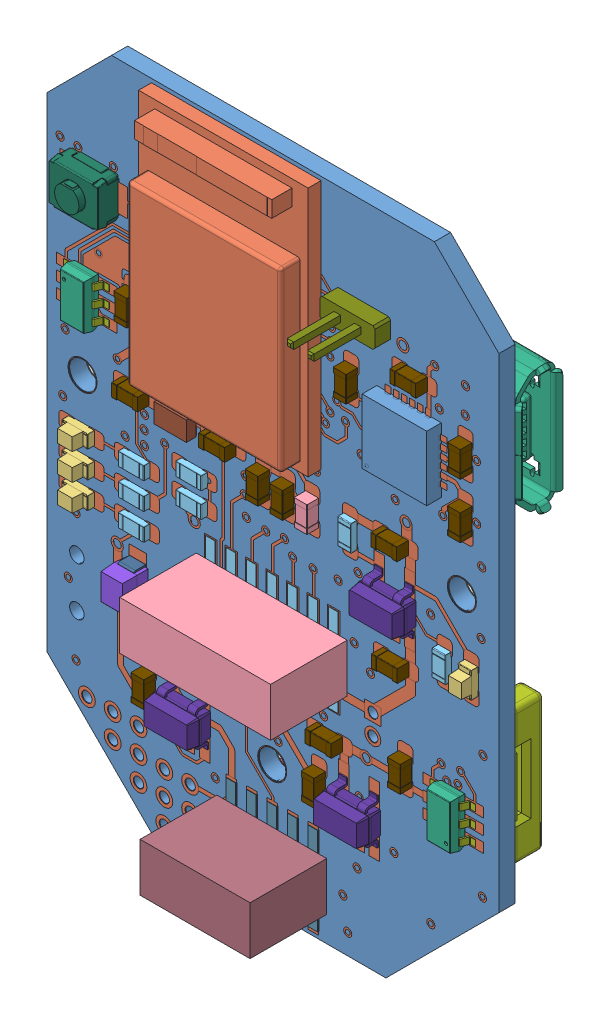
SolidWorks assembly mainboard, configuration Default. Lengths in mm.
Overall size (28.95 41 10.7).
78 component instances, 27 part files, 2 mates.
Components (placement in the parent):
- Board_Geoms_6845.step-1: Board_Geoms_6845.step [Default] at origin size (28 41 1.11)
  - Pcb_6845.step-1: Pcb_6845.step [Default] at (-183 131 0) size (28 41 1)
  - topTracks_6845.step-1: topTracks_6845.step [Default] at (-183 131 0.01) size (26.72 36.74 0.06)
  - botTracks_6845.step-1: botTracks_6845.step [Default] at (-183 131 -1.01) size (26.97 36.83 0.05)
- components_6845.step-1: components_6845.step [Default] at (0 0 -0.0254) size (28.75 40.34 10.7)
  - Top_6845.step-1: Top_6845.step [Default] at origin size (25.79 40.34 7.15)
    - J6_ASSEMBLY_6124D9AA.step-1: J6_ASSEMBLY_6124D9AA.step [Default] at (7 15.5 0) size (9.35 5.45 4.85)
      - Body.step-1: Body.step [Default] at (0 0 0.1) size (9.35 3 4.75)
      - Pins.step-1: Pins.step [Default] at origin size (8.23 5.45 0.1)
    - IC2_ASSEMBLY_61243599.step-1: IC2_ASSEMBLY_61243599.step [Default] at (18.21 11 0) x (-1 0 0) z (0 0 1) size (2.8 2.9 1)
      - Body001.step-1: Body001.step [Default] at origin size (1.6 2.9 0.95)
      - PinsArrayLR.step-1: PinsArrayLR.step [Default] at origin size (2.8 2.3 0.54)
    - IC2_ASSEMBLY_61243599.step-2: IC2_ASSEMBLY_61243599.step [Default] at (-4.49 27.54 0) size (2.8 2.9 1)
      - Body001.step-1: Body001.step [Default] at origin size (1.6 2.9 0.95)
      - PinsArrayLR.step-1: PinsArrayLR.step [Default] at origin size (2.8 2.3 0.54)
    - C13_ASSEMBLY_61236D87.step-1: C13_ASSEMBLY_61236D87.step [Default] at (-1.32 13.77 0) x (0 1 0) z (0 0 1) size (2.05 1.4 1.7)
      - Body002.step-1: Body002.step [Default] at origin size (1.85 1.4 1.6)
      - FilletPin1.step-1: FilletPin1.step [Default] at origin size (0.6 1 0.82)
      - FilletPin2.step-1: FilletPin2.step [Default] at origin size (0.7 1 0.82)
    - XTAL1_ASSEMBLY_611ED8A0.step-1: XTAL1_ASSEMBLY_611ED8A0.step [Default] at (1.31 23.82 0) size (2 1.2 0.7)
      - Body003.step-1: Body003.step [Default] at (0 0 0.1) size (2 1.2 0.6)
      - Pins001.step-1: Pins001.step [Default] at origin size (1.88 0.98 0.1)
    - J7_ASSEMBLY_612472BA[2].step-1: J7_ASSEMBLY_612472BA[2].step [Default] at (7 3.15 0) size (6.81 5.45 4.85)
      - Body004.step-1: Body004.step [Default] at (0 0 0.1) size (6.81 3 4.75)
      - Pins002.step-1: Pins002.step [Default] at origin size (5.69 5.45 0.1)
    - S1_B3U-1000P_6128C187.step-1: S1_B3U-1000P_6128C187.step [Default] at (-4.05 33.62 0) x (1 0 0) z (0 -1 0) size (4 1.75 2.5)
    - J4_PinHeader_2x01_P127mm_Vertical_6123D488.step-1: J4_PinHeader_2x01_P127mm_Vertical_6123D488.step [Default] at (11.96 34.93 0) size (3.4 1.27 6.3)
    - U7_SOT_23_5_61231905.step-1: U7_SOT_23_5_61231905.step [Default] at (12.38 8.22 0) x (0 1 0) z (0 0 1) size (2.8 2.9 1.55)
    - C18_C_0603_1608Metric_61231302.step-1: C18_C_0603_1608Metric_61231302.step [Default] at (9.91 8.45 0) x (0 -1 0) z (0 0 1) size (1.6 0.8 0.8)
    - C18_C_0603_1608Metric_61231302.step-2: C18_C_0603_1608Metric_61231302.step [Default] at (10.57 11.24 0) size (1.6 0.8 0.8)
    - C18_C_0603_1608Metric_61231302.step-3: C18_C_0603_1608Metric_61231302.step [Default] at (14.67 17.31 0) size (1.6 0.8 0.8)
    - C18_C_0603_1608Metric_61231302.step-4: C18_C_0603_1608Metric_61231302.step [Default] at (14.64 23.82 0) size (1.6 0.8 0.8)
    - C18_C_0603_1608Metric_61231302.step-5: C18_C_0603_1608Metric_61231302.step [Default] at (7.96 22.91 0) x (0 1 0) z (0 0 1) size (1.6 0.8 0.8)
    - C18_C_0603_1608Metric_61231302.step-6: C18_C_0603_1608Metric_61231302.step [Default] at (-1.69 28.4 0) x (0 -1 0) z (0 0 1) size (1.6 0.8 0.8)
    - C18_C_0603_1608Metric_61231302.step-7: C18_C_0603_1608Metric_61231302.step [Default] at (15.25 11.86 0) x (0 -1 0) z (0 0 1) size (1.6 0.8 0.8)
    - U5_MPU-6050_61201B19.step-1: U5_MPU-6050_61201B19.step [Default] at (15.43 29.5 0) x (0 1 0) z (1 0 0) size (4 0.95 4)
    - C18_C_0603_1608Metric_61231302.step-8: C18_C_0603_1608Metric_61231302.step [Default] at (11.9 31.11 0) x (0 -1 0) z (0 0 1) size (1.6 0.8 0.8)
    - C18_C_0603_1608Metric_61231302.step-9: C18_C_0603_1608Metric_61231302.step [Default] at (18.98 30.62 0) x (0 -1 0) z (0 0 1) size (1.6 0.8 0.8)
    - C18_C_0603_1608Metric_61231302.step-10: C18_C_0603_1608Metric_61231302.step [Default] at (18.98 27.22 0) x (0 1 0) z (0 0 1) size (1.6 0.8 0.8)
    - C18_C_0603_1608Metric_61231302.step-11: C18_C_0603_1608Metric_61231302.step [Default] at (15.81 33.18 0) size (1.6 0.8 0.8)
    - U7_SOT_23_5_61231905.step-2: U7_SOT_23_5_61231905.step [Default] at (1.86 8.23 0) x (0 1 0) z (0 0 1) size (2.8 2.9 1.55)
    - U7_SOT_23_5_61231905.step-3: U7_SOT_23_5_61231905.step [Default] at (14.58 20.54 0) x (0 1 0) z (0 0 1) size (2.8 2.9 1.55)
    - U1_MDBT50Q-1MV2_611EF495.step-1: U1_MDBT50Q-1MV2_611EF495.step [Default] at (4.3136 32.395 0.0254) x (-1 0 0) z (0 1 0) size (10.5 2.06 15.5)
    - C18_C_0603_1608Metric_61231302.step-12: C18_C_0603_1608Metric_61231302.step [Default] at (6.44 22.91 0) x (0 1 0) z (0 0 1) size (1.6 0.8 0.8)
    - C18_C_0603_1608Metric_61231302.step-13: C18_C_0603_1608Metric_61231302.step [Default] at (-1.43 23.82 0) x (-1 0 0) z (0 0 1) size (1.6 0.8 0.8)
    - C18_C_0603_1608Metric_61231302.step-14: C18_C_0603_1608Metric_61231302.step [Default] at (3.97 23.82 0) size (1.6 0.8 0.8)
    - C18_C_0603_1608Metric_61231302.step-15: C18_C_0603_1608Metric_61231302.step [Default] at (1.77 11.25 0) x (-1 0 0) z (0 0 1) size (1.6 0.8 0.8)
    - C18_C_0603_1608Metric_61231302.step-16: C18_C_0603_1608Metric_61231302.step [Default] at (-0.63 8.46 0) x (0 -1 0) z (0 0 1) size (1.6 0.8 0.8)
    - D1_LED_0603_1608Metric_611ED4CA.step-1: D1_LED_0603_1608Metric_611ED4CA.step [Default] at (-4.81 19.99 0) size (1.6 0.8 1.1)
    - D1_LED_0603_1608Metric_611ED4CA.step-2: D1_LED_0603_1608Metric_611ED4CA.step [Default] at (-4.81 18.34 0) size (1.6 0.8 1.1)
    - D1_LED_0603_1608Metric_611ED4CA.step-3: D1_LED_0603_1608Metric_611ED4CA.step [Default] at (-4.81 16.69 0) size (1.6 0.8 1.1)
    - D1_LED_0603_1608Metric_611ED4CA.step-4: D1_LED_0603_1608Metric_611ED4CA.step [Default] at (19.34 18.79 0) x (0 1 0) z (0 0 1) size (1.6 0.8 1.1)
    - L1_L_0603_1608Metric_611ED393.step-1: L1_L_0603_1608Metric_611ED393.step [Default] at (9.48 22.91 0) x (0 1 0) z (0 0 1) size (1.6 0.8 0.8)
    - R11_R_0603_1608Metric_6124489D.step-1: R11_R_0603_1608Metric_6124489D.step [Default] at (2.18 19.69 0) x (-1 0 0) z (0 0 1) size (1.6 0.8 0.45)
    - R11_R_0603_1608Metric_6124489D.step-2: R11_R_0603_1608Metric_6124489D.step [Default] at (2.18 21.23 0) size (1.6 0.8 0.45)
    - R11_R_0603_1608Metric_6124489D.step-3: R11_R_0603_1608Metric_6124489D.step [Default] at (-1.38 19.99 0) size (1.6 0.8 0.45)
    - R11_R_0603_1608Metric_6124489D.step-4: R11_R_0603_1608Metric_6124489D.step [Default] at (-1.38 18.34 0) size (1.6 0.8 0.45)
    - R11_R_0603_1608Metric_6124489D.step-5: R11_R_0603_1608Metric_6124489D.step [Default] at (-1.38 16.69 0) x (-1 0 0) z (0 0 1) size (1.6 0.8 0.45)
    - R11_R_0603_1608Metric_6124489D.step-6: R11_R_0603_1608Metric_6124489D.step [Default] at (11.84 22.9 0) x (0 1 0) z (0 0 1) size (1.6 0.8 0.45)
    - R11_R_0603_1608Metric_6124489D.step-7: R11_R_0603_1608Metric_6124489D.step [Default] at (17.69 18.7675 0) x (0 1 0) z (0 0 1) size (1.6 0.8 0.45)
  - Bot_6845.step-1: Bot_6845.step [Default] at origin size (28.75 36.79 5.35)
    - C13_ASSEMBLY_61236D87.step-1: C13_ASSEMBLY_61236D87.step [Default] at (13.22 32.86 -1) x (-1 0 0) z (0 0 -1) size (2.05 1.4 1.7)
      - Body002.step-1: Body002.step [Default] at origin size (1.85 1.4 1.6)
      - FilletPin1.step-1: FilletPin1.step [Default] at origin size (0.6 1 0.82)
      - FilletPin2.step-1: FilletPin2.step [Default] at origin size (0.7 1 0.82)
    - J7_ASSEMBLY_612472BA[2].step-1: J7_ASSEMBLY_612472BA[2].step [Default] at (7 3.15 -1) x (1 0 0) z (0 0 -1) size (6.81 5.45 4.85)
      - Body004.step-1: Body004.step [Default] at (0 0 0.1) size (6.81 3 4.75)
      - Pins002.step-1: Pins002.step [Default] at origin size (5.69 5.45 0.1)
    - J2_473460001_61208B11.step-1: J2_473460001_61208B11.step [Default] at (18.68 31.28 -2.2) x (0 -1 0) z (1 0 0) size (4 2.15 2.5)
      - SOLID.step-1: SOLID.step [Default] at origin size (1.6 0.8 0.45)
      - COMPOUND.step-1: COMPOUND.step [Default] at origin size (4 1.75 2.5)
    - R11_R_0603_1608Metric_6124489D.step-1: R11_R_0603_1608Metric_6124489D.step [Default] at (12.55 26.62 -1) x (1 0 0) z (0 0 -1) size (1.6 0.8 0.45)
    - R11_R_0603_1608Metric_6124489D.step-2: R11_R_0603_1608Metric_6124489D.step [Default] at (9.6 31.14 -1) x (0 1 0) z (0 0 -1) size (1.6 0.8 0.45)
    - J8_1734592-6_61209AA8.step-1: J8_1734592-6_61209AA8.step [Default] at (20.79 13 -2) x (0 -1 0) z (1 0 0) size (8.43 2.05 5.11)
    - J8_1734592-6_61209AA8.step-2: J8_1734592-6_61209AA8.step [Default] at (-6.81 33 -2) x (0 1 0) z (-1 0 0) size (8.43 2.05 5.11)
    - R11_R_0603_1608Metric_6124489D.step-3: R11_R_0603_1608Metric_6124489D.step [Default] at (13.22 29.49 -1) x (-1 0 0) z (0 0 -1) size (1.6 0.8 0.45)
    - R11_R_0603_1608Metric_6124489D.step-4: R11_R_0603_1608Metric_6124489D.step [Default] at (13.22 31.0275 -1) x (-1 0 0) z (0 0 -1) size (1.6 0.8 0.45)
    - SW1_Fusion_sp_611ED265.step-1: SW1_Fusion_sp_611ED265.step [Default] at (-4.82 11.63 -1) x (0 1 0) z (0 0 -1) size (7.7 5 2)
Mates (geometry in assembly coordinates):
- Coincident1: coincident anti-aligned: plane of Board_Geoms_6845.step-1/Pcb_6845.step-1 through (7 21.1851 0) normal (0 0 1); plane of components_6845.step-1/Top_6845.step-1/U1_MDBT50Q-1MV2_611EF495.step-1 through (4.3136 32.395 0) normal (0 0 -1)
- Concentric1: concentric anti-aligned: cylinder of Board_Geoms_6845.step-1/Pcb_6845.step-1 through (-5.15 13.13 0) axis (0 0 1) radius 0.45; cylinder of components_6845.step-1/Bot_6845.step-1/SW1_Fusion_sp_611ED265.step-1 through (-5.15 13.13 -0.5254) axis (0 0 -1) radius 0.4
